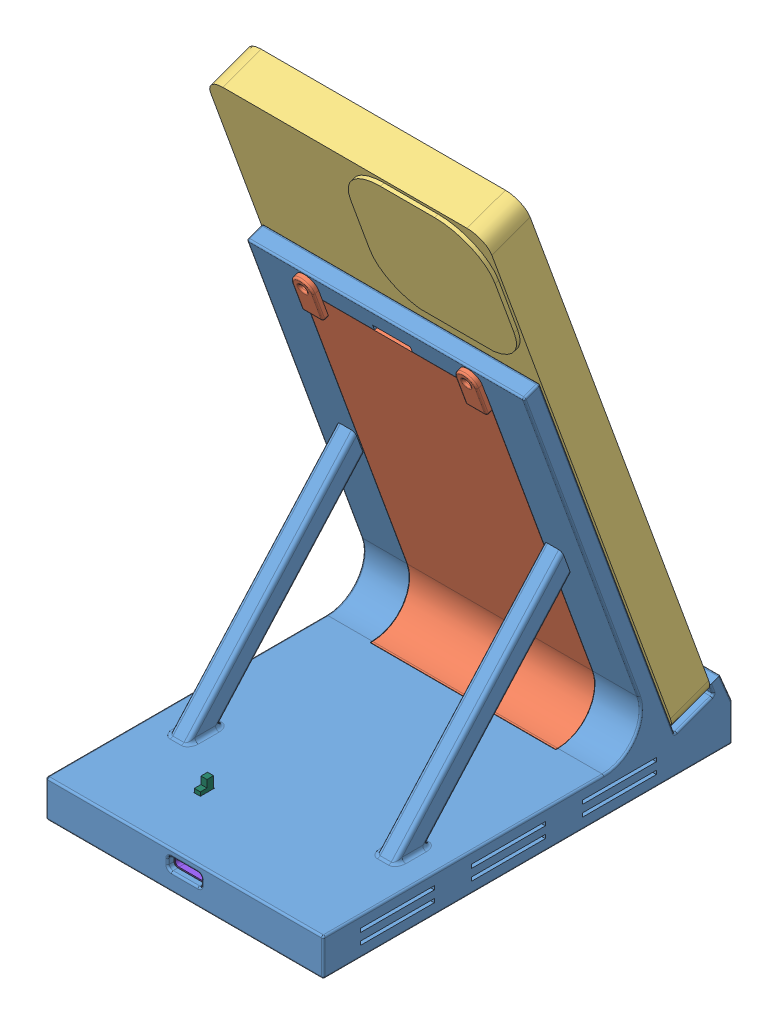
SolidWorks assembly IP支架装配体_配重块, configuration 默认. Lengths in mm.
Overall size (76 155.66 111.5).
31 component instances, 16 part files, 25 mates.
Components (placement in the parent):
- IP支架-1: IP支架 [默认] at (-19.3867 -35.6954 110) size (75 110.1 110.5)
- IP线圈支架零件-1: IP线圈支架零件 [默认] at (-19.3867 -31.7451 120.1792) x (0 0 -1) z (1 0 0) size (35.67 101.03 50)
- IP手机-1: IP手机 [默认] at (-19.3867 45.2514 95.8225) x (1 0 0) z (0 0.939693 0.34202) size (76 12 151)
- 充电线圈-1: 充电线圈 [默认] at (-19.3867 43.7507 97.2983) x (1 0 0) z (0 -0.939693 -0.34202) size (43 1.52 55.03)
- 充电零件板-1: 充电零件板 [默认] at (-19.3867 -32.5954 114.2877) x (-1 0 0) z (0 0 -1) size (21 2 28)
- IP底板-1: IP底板 [默认] at (-35.435 -35.6954 107.1856) x (0 0 -1) z (1 0 0) size (102.06 4.25 64.8)
- TypeC电路板-2: TypeC电路板 [默认] at (2.6105 -32.1554 166.4993) x (0 0 -1) z (0 1 0) size (30 34.97 13.16)
  - TypeC电路板.STEP-1: TypeC电路板.STEP [默认] at origin size (30 34.97 13.16)
    - TypeC______.STEP.STEP-1: TypeC______.STEP.STEP [默认] at origin size (30 34.97 13.16)
      - 5v06-R1.STEP.STEP-1: 5v06-R1.STEP.STEP [默认] at (25.0953 30.8357 1.2) x (-1 0 0) z (0 0 1) size (2 1.3 0.61)
        - R0805.STEP.STEP-1: R0805.STEP.STEP [默认] at origin size (2 1.3 0.61)
          - COMPOUND.STEP.STEP-1: COMPOUND.STEP.STEP [默认] at origin size (2 1.3 0.61)
      - 5v06-USB1.STEP.STEP-1: 5v06-USB1.STEP.STEP [默认] at (8.1992 21.9972 1.2) x (0 -1 0) z (0 0 1) size (8.95 7.58 4.16)
        - USB-C-SMD_TYPE-C-6PIN-2MD-073.STEP.STEP-1: USB-C-SMD_TYPE-C-6PIN-2MD-073.STEP.STEP [默认] at origin size (8.95 7.58 4.16)
          - COMPOUND-1.STEP.STEP-1: COMPOUND-1.STEP.STEP [默认] at origin size (8.95 7.58 4.16)
      - 5v06-U2.STEP.STEP-1: 5v06-U2.STEP.STEP [默认] at (19.685 34.9251 0) x (-1 0 0) z (0 0 -1) size (8.51 3.81 11.5) (hidden)
        - SW-TH_DEALON_SS-12D01-GX.STEP.STEP-1: SW-TH_DEALON_SS-12D01-GX.STEP.STEP [默认] at origin size (8.51 3.81 11.5)
          - COMPOUND-2.STEP.STEP-1: COMPOUND-2.STEP.STEP [默认] at origin size (8.51 3.81 11.5)
      - 5v06-C1.STEP.STEP-1: 5v06-C1.STEP.STEP [默认] at (18.2118 28.8799 1.2) size (3.2 2.52 0.9)
        - C1210.STEP.STEP-1: C1210.STEP.STEP [默认] at origin size (3.2 2.52 0.9)
          - SOLID-3.STEP.STEP-1: SOLID-3.STEP.STEP [默认] at origin size (3.2 2.52 0.9)
      - 5v06-C2.STEP.STEP-1: 5v06-C2.STEP.STEP [默认] at (24.13 13.843 1.2) x (0 1 0) z (0 0 1) size (1.6 0.8 0.8)
        - C0603.STEP.STEP-1: C0603.STEP.STEP [默认] at origin size (1.6 0.8 0.8)
          - SOLID-4.STEP.STEP-1: SOLID-4.STEP.STEP [默认] at origin size (1.6 0.8 0.8)
      - 5v06-U4.STEP.STEP-1: 5v06-U4.STEP.STEP [默认] at (18.386 14.645 1.2) size (4.1 4.3 1.61)
        - SOT-89-3_L4.5-W2.5-P1.50-LS4.2-BR.STEP.STEP-1: SOT-89-3_L4.5-W2.5-P1.50-LS4.2-BR.STEP.STEP [默认] at origin size (4.1 4.3 1.61)
          - SOLID-5.STEP.STEP-1: SOLID-5.STEP.STEP [默认] at origin size (4.1 4.3 1.61)
      - Board.STEP.STEP-1: Board.STEP.STEP [默认] at origin size (29.97 34.97 1.2)
- Led5mmRojo_.step-1: Led5mmRojo_.step [默认] at (-19.3867 -30.9454 79) x (0 0 -1) z (1 0 0) size (25.5 5.8 5.4)
- 配重块-1: 配重块 [默认] at (-19.3867 -34.1954 110) x (0 0 1) z (-1 0 0) size (92 1.6 50)
- 开关-1: 开关 [默认] at (-32.324 -30.7554 146.8123) x (0 0 1) z (-1 0 0) size (8.5 11.2 3.5)
Mates (geometry in assembly coordinates):
- 重合1: coincident anti-aligned: plane of IP支架-1 through (126.3422 74.5456 106.4847) normal (0 0.34202 -0.939693); plane of IP手机-1 through (-19.3867 45.2514 95.8225) normal (0 -0.34202 0.939693)
- 宽度1: width aligned: plane of IP支架-1 through (18.1133 -25.6954 165) normal (1 0 0); plane of IP手机-1 through (-56.8867 -25.6954 165) normal (-1 0 0); plane of IP支架-1 through (18.6133 -21.9332 59.6634) normal (1 0 0); plane of IP手机-1 through (-57.3867 -21.9332 59.6634) normal (-1 0 0)
- 重合8: coincident anti-aligned: plane of IP线圈支架零件-1 through (-19.3867 43.2377 98.7078) normal (0 0.34202 -0.939693); plane of 充电线圈-1 through (-19.3867 43.2377 98.7078) normal (0 -0.34202 0.939693)
- 同心1: concentric aligned: cylinder of IP线圈支架零件-1 through (-19.3867 43.2377 98.7078) axis (0 0.34202 -0.939693) radius 22; cylinder of 充电线圈-1 through (-19.3867 43.2377 98.7078) axis (0 0.34202 -0.939693) radius 21.5
- 重合15: coincident aligned: plane of IP线圈支架零件-1 through (-19.3867 -31.7451 120.1792) normal (1 0 0); plane of 充电线圈-1 through (-19.3867 43.7507 97.2983) normal (1 0 0)
- 宽度11: width anti-aligned: plane of IP支架-1 through (-400019.3867 -35.6964 159) normal (0 0 -1); plane of IP支架-1 through (-400019.3867 -35.6964 61) normal (0 0 1); plane of IP底板-1 through (-51.7867 -34.1954 158.9) normal (0 0 1); plane of IP底板-1 through (-51.7867 -34.1954 61.1) normal (0 0 -1)
- 重合52: coincident anti-aligned: plane of IP支架-1 through (-80.3851 -25.6954 70) normal (0 0.939693 0.34202); plane of IP手机-1 through (-57.3867 -21.9332 59.6634) normal (0 -0.939693 -0.34202)
- 宽度17: width: plane of IP支架-1 through (18.1133 -25.6954 165) normal (1 0 0); plane of IP支架-1 through (-56.8867 -25.6954 165) normal (-1 0 0); cylinder of Led5mmRojo_.step-1 through (-19.3867 -30.9454 61) axis (0 0 -1) radius 2.5
- 平行1: parallel aligned: plane of IP支架-1 through (-19.3867 -35.6954 110) normal (0 -1 0); plane of Led5mmRojo_.step-1 through (-18.3667 -31.1954 62) normal (0 -1 0)
- 重合55: coincident anti-aligned: plane of IP支架-1 through (-400019.3867 -35.6964 61) normal (0 0 1); plane of Led5mmRojo_.step-1 through (-19.1867 -30.9454 61) normal (0 0 -1)
- 宽度18: width aligned: plane of IP底板-1 through (-51.7867 -34.1954 158.9) normal (-1 0 0); plane of IP底板-1 through (13.0133 -34.1954 158.9) normal (1 0 0); plane of 配重块-1 through (-44.3867 -32.5954 64) normal (-1 0 0); plane of 配重块-1 through (5.6133 -32.5954 64) normal (1 0 0)
- 距离1: distance = 0.2 mm anti-aligned: plane of 开关-1 through (-32.324 -30.7554 146.8123) normal (0 -1 0); plane of TypeC电路板-2/TypeC电路板.STEP-1/TypeC______.STEP.STEP-1/Board.STEP.STEP-1 through (-19.3867 -30.9554 146.9463) normal (0 1 0)
- 距离2: distance = 2.8 mm aligned: plane of 开关-1 through (-34.074 -26.7554 142.5623) normal (-1 0 0); plane of TypeC电路板-2/TypeC电路板.STEP-1/TypeC______.STEP.STEP-1/Board.STEP.STEP-1 through (-36.874 -32.1554 155.7623) normal (-1 0 0)
- 距离3: distance = 4.7 mm aligned: plane of 开关-1 through (-30.574 -26.7554 151.0623) normal (0 0 1); plane of TypeC电路板-2/TypeC电路板.STEP-1/TypeC______.STEP.STEP-1/Board.STEP.STEP-1 through (-25.3867 -32.1554 155.7623) normal (0 0 1)
- 重合60: coincident anti-aligned: plane of IP支架-1 through (-19.3867 -27.6954 110) normal (0 -1 0); plane of TypeC电路板-2/TypeC电路板.STEP-1/TypeC______.STEP.STEP-1/5v06-USB1.STEP.STEP-1/USB-C-SMD_TYPE-C-6PIN-2MD-073.STEP.STEP-1/COMPOUND-1.STEP.STEP-1 through (-22.6068 -27.6954 155.96) normal (0 1 0)
- 宽度19: width anti-aligned: plane of IP支架-1 through (-51.8867 -35.6964 291654.25) normal (1 0 0); plane of TypeC电路板-2/TypeC电路板.STEP-1/TypeC______.STEP.STEP-1/Board.STEP.STEP-1 through (13.1133 -35.6964 291654.25) normal (-1 0 0); plane of IP支架-1 through (-36.874 -32.1554 155.7623) normal (-1 0 0); plane of TypeC电路板-2/TypeC电路板.STEP-1/TypeC______.STEP.STEP-1/Board.STEP.STEP-1 through (-1.8994 -32.1554 133.2877) normal (1 0 0)
- 重合61: coincident anti-aligned: plane of IP支架-1 through (-400019.3867 -35.6964 163.2623) normal (0 0 -1); plane of TypeC电路板-2/TypeC电路板.STEP-1/TypeC______.STEP.STEP-1/Board.STEP.STEP-1 through (-13.3994 -32.1554 163.2623) normal (0 0 1)
- 宽度21: width anti-aligned: plane of IP支架-1 through (-400019.3867 -35.6964 159) normal (0 0 -1); plane of 配重块-1 through (-400019.3867 -35.6964 61) normal (0 0 1); plane of IP支架-1 through (5.6133 -32.5954 156) normal (0 0 1); plane of 配重块-1 through (5.6133 -32.5954 64) normal (0 0 -1)
- 重合62: coincident anti-aligned: plane of 充电零件板-1 through (-17.3867 -32.5954 108.6627) normal (0 -1 0); plane of 配重块-1 through (-19.3867 -32.5954 110) normal (0 1 0)
- 距离4: distance = 5 mm anti-aligned: plane of 充电零件板-1 through (-11.3867 -30.5954 128.2877) normal (0 0 1); plane of TypeC电路板-2/TypeC电路板.STEP-1/TypeC______.STEP.STEP-1/Board.STEP.STEP-1 through (-36.874 -32.1554 133.2877) normal (0 0 -1)
- 重合63: coincident anti-aligned: plane of IP底板-1 through (-35.435 -34.1954 107.1856) normal (0 1 0); plane of 配重块-1 through (-19.3867 -34.1954 110) normal (0 -1 0)
- 宽度23: width aligned: plane of IP底板-1 through (-51.7867 -34.1954 158.9) normal (-1 0 0); plane of IP底板-1 through (13.0133 -34.1954 158.9) normal (1 0 0); plane of 充电零件板-1 through (-29.8867 -30.5954 125.2877) normal (-1 0 0); plane of 充电零件板-1 through (-8.8867 -30.5954 125.2877) normal (1 0 0)
- 宽度24: width anti-aligned: plane of IP支架-1 through (-51.8867 -35.6964 291654.25) normal (1 0 0); plane of IP支架-1 through (13.1133 -35.6964 291654.25) normal (-1 0 0); plane of IP底板-1 through (-51.7867 -34.1954 158.9) normal (-1 0 0); plane of IP底板-1 through (13.0133 -34.1954 158.9) normal (1 0 0)
- 重合64: coincident aligned: plane of IP支架-1 through (-19.3867 -35.6954 110) normal (0 -1 0); plane of IP底板-1 through (-35.435 -35.6954 107.1856) normal (0 -1 0)
- 宽度25: width: plane of IP支架-1 through (-19.3867 -27.6954 110) normal (0 -1 0); plane of IP底板-1 through (-35.435 -34.1954 107.1856) normal (0 1 0); cylinder of Led5mmRojo_.step-1 through (-19.3867 -30.9454 61) axis (0 0 -1) radius 2.5
